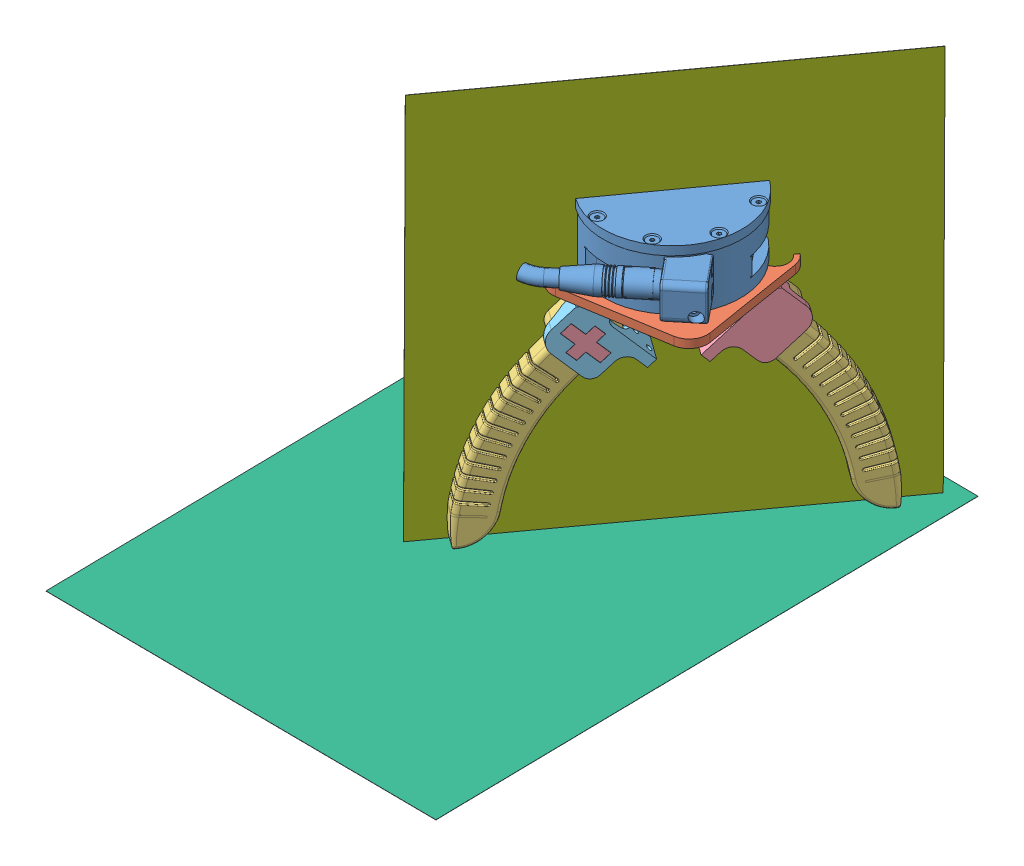
SolidWorks assembly Assem_ee, configuration Default. Lengths in mm.
Overall size (212.48 223.84 298.79).
58 component instances, 34 part files, 23 mates.
Components (placement in the parent):
- ati_gamma_sensor_mount _up-1: ati_gamma_sensor_mount _up [Default] at (-15.434 18.2375 114.8285) size (94 14.49 94) (hidden)
- ati_gamma_sensor_mount _down_L515-1: ati_gamma_sensor_mount _down_L515 [Default] at (-15.434 18.2375 114.8285) x (0 0 1) z (-1 0 0) size (114.18 58 114.18) (hidden)
- ATI-9105-TIF-GAMMA-1: ATI-9105-TIF-GAMMA [Default] at (-15.434 10.2375 114.8285) x (-0.987109 0 0.160048) z (0 1 0) size (81.43 106.62 33.32)
- fixture-1: fixture [Default] at (15.9943 -30.0869 71.2365) x (-0.987109 0 0.160048) z (0 1 0) size (76 76 7.57)
- Assem_soft-1: Assem_soft [Default] at (-95.8769 -63.8673 78.8152) x (0.181198 -0.950797 -0.251303) z (0.811158 0.000013 0.584827) size (139.54 63.23 30.2)
  - finger_proto_4.2-1: finger_proto_4.2 [Default] at (-2.494 64.561 95.5128) size (120.36 42.19 26.68)
  - linkag_3-1: linkag_3 [Default] at (-2.8273 57.773 71.3134) x (0.891388 0.453242 -0.000014) z (0.000014 0.000003 1) size (40.75 42 30.2)
  - linkage_4-1: linkage_4 [Default] at (-2.8273 57.773 71.3134) x (0.891388 0.453242 -0.000014) z (0.000014 0.000003 1) size (40.75 42 15)
- Assem_soft-2: Assem_soft [Default] at (65.1711 -63.8673 150.9587) x (-0.181198 -0.950797 0.251303) z (-0.811158 0.000013 -0.584827) size (139.54 63.23 30.2)
  - finger_proto_4.2-1: finger_proto_4.2 [Default] at (-2.494 64.561 95.5128) size (120.36 42.19 26.68)
  - linkag_3-1: linkag_3 [Default] at (-2.8273 57.773 71.3134) x (0.891388 0.453242 -0.000014) z (0.000014 0.000003 1) size (40.75 42 30.2)
  - linkage_4-1: linkage_4 [Default] at (-2.8273 57.773 71.3134) x (0.891388 0.453242 -0.000014) z (0.000014 0.000003 1) size (40.75 42 15)
- Assem1-1: Assem1 [Default] at (17.137 -120.8618 -18.1601) x (0.539853 0.425322 0.726403) z (-0.534722 0.839751 -0.094291) size (112.36 145.16 142) (hidden)
  - CAM holder (1)-1: CAM holder (1) [Default] at (82.7281 3.9301 79.7737) x (0.895378 -0.021687 -0.444779) z (0.425322 0.33752 0.839751) size (64.99 120.47 90)
  - Top CAM (1)-1: Top CAM (1) [Default] at (81.9279 129.0526 71.921) x (0.895378 -0.021687 -0.444779) z (-0.425322 -0.33752 -0.839751) size (65 111.17 15.1)
- Intel_RealSense_L515_CAD_external.stp-1: Intel_RealSense_L515_CAD_external.stp [Default] at (106.8055 -15.7625 -7.3222) x (-0.587716 0 -0.809067) z (0 -1 0) size (61.01 64.04 35.39) (hidden)
  - TA_PERIPHERAL_L515_ASM_25_ASM.stp-1: TA_PERIPHERAL_L515_ASM_25_ASM.stp [Default] at origin size (61.01 64.04 35.39)
    - CENTER_HEAT_SINK_SUBASM_L515_AS_ASM.stp-1: CENTER_HEAT_SINK_SUBASM_L515_AS_ASM.stp [Default] at origin size (26.06 28.22 15.92)
      - OPTICAL_HEAD_GEN_1_L515_ASM_6_ASM.stp-1: OPTICAL_HEAD_GEN_1_L515_ASM_6_ASM.stp [Default] at origin size (26.06 28.22 15.92)
        - RXFOV_72X60_P_040419_2.stp-1: RXFOV_72X60_P_040419_2.stp [Default] at (-18.5 -15 -9.623) size (26.06 21.31 15.92) (hidden)
        - TX_FOV_1_2_73X59_040419_2.stp-1: TX_FOV_1_2_73X59_040419_2.stp [Default] at (-18.5 -15 -9.623) size (19.97 16.11 9.45) (hidden)
    - FRONT_OPTICAL_ASSEMBLY_L515_ASM_ASM.stp-1: FRONT_OPTICAL_ASSEMBLY_L515_ASM_ASM.stp [Default] at origin size (24.45 11.78 6.27)
      - CAMERA_2MP_FF_OV2740_CMOS_ASM_1_ASM.stp-1: CAMERA_2MP_FF_OV2740_CMOS_ASM_1_ASM.stp [Default] at (0 0 -22.68) size (8 5.7 2.8)
        - L500_RGB_2MP_1_2_2.stp-1: L500_RGB_2MP_1_2_2.stp [Default] at origin size (8 5.7 2.8)
      - PCB_ASSY_RGB_INTERPOSER_L515_AS_ASM.stp-1: PCB_ASSY_RGB_INTERPOSER_L515_AS_ASM.stp [Default] at origin size (24.45 11.78 3.75)
        - RGB_INTERPOSER_AS03021_23AUG_7.stp-1: RGB_INTERPOSER_AS03021_23AUG_7.stp [Default] at (-14.55 7.36 -5.546) size (24.45 11.78 3.72)
        - KAPTON_RGB_INTERPOSER_L515_8.stp-1: KAPTON_RGB_INTERPOSER_L515_8.stp [Default] at origin size (20.84 11.78 0.05)
        - CONN_FPC_BTM_21POS_-3MM_PITCH_2.stp-1: CONN_FPC_BTM_21POS_-3MM_PITCH_2.stp [Default] at (11.985 13.432 -5.615) x (0 -1 0) z (1 0 0) size (7.5 0.9 2.83)
        - CONN_HEADER_3-0MM_20POS_PWR_2.stp-1: CONN_HEADER_3-0MM_20POS_PWR_2.stp [Default] at (-10.26 11.36 -5.58) x (0 -1 0) z (0 0 -1) size (5.9 2.35 2.24)
    - PCB_ASSEMBLY_MA_ASIC_L515_ASM_5_ASM.stp-1: PCB_ASSEMBLY_MA_ASIC_L515_ASM_5_ASM.stp [Default] at origin size (43.47 31.41 6.28)
      - L500_PCB_ASIC_BOARD_OCT08_ASM_1_ASM.stp-1: L500_PCB_ASIC_BOARD_OCT08_ASM_1_ASM.stp [Default] at (0 0 0.6) size (43.47 31.41 6.28)
        - A-PCB_ASIC_20_ASM_1_ASM_1_ASM.stp-1: A-PCB_ASIC_20_ASM_1_ASM_1_ASM.stp [Default] at origin size (43.47 31.41 6.28)
          - 2UB2C02-000111F_3D_USB_TYPE_C_1_ASM.stp-1: 2UB2C02-000111F_3D_USB_TYPE_C_1_ASM.stp [Default] at (-14.4895 -10.5138 -15.4) x (-0.58723 0.80942 0) z (0 0 -1) size (9.7 11.1 6.08)
            - 2UB2C02-000111F_3D_USB_TYPE_C_2.stp-1: 2UB2C02-000111F_3D_USB_TYPE_C_2.stp [Default] at origin size (9.7 11.1 6.08)
            - 2UB2C02-000111F_3D_USB_TYPE_C_3.stp-1: 2UB2C02-000111F_3D_USB_TYPE_C_3.stp [Default] at origin size (0.28 0.35 0.16)
          - P-PCB_ASIC_20_1_3.stp-1: P-PCB_ASIC_20_1_3.stp [Default] at origin size (41.95 30.8 1)
      - BM03B-SRSS-TB_1.stp-1: BM03B-SRSS-TB_1.stp [Default] at (15.2095 -11.0504 -16.2) x (0.587785 0.809017 0) z (0 0 -1) size (5 4.32 3.6)
    - REAR_HOUSING_ASSEMBLY_L515_ASM__ASM.stp-1: REAR_HOUSING_ASSEMBLY_L515_ASM__ASM.stp [Default] at origin size (61.01 64.04 26)
      - INTAKE_VENT_L515_9.stp-1: INTAKE_VENT_L515_9.stp [Default] at origin size (12.82 7.66 16.91)
      - INTAKE_VENT_L515_9.stp-2: INTAKE_VENT_L515_9.stp [Default] x (0.660526 0.750803 0) z (0 0 1) size (12.82 7.66 16.91)
      - REAR_HOUSING_L515_25.stp-1: REAR_HOUSING_L515_25.stp [Default] at origin size (61.01 61.01 26)
    - COVER_WINDOW_SUBASM_L515_ASM_2_ASM.stp-1: COVER_WINDOW_SUBASM_L515_ASM_2_ASM.stp [Default] at origin size (57.86 57.86 2.18)
      - COVER_WINDOW_IR_W_ADHESIVE_L515_ASM.stp-1: COVER_WINDOW_IR_W_ADHESIVE_L515_ASM.stp [Default] at origin size (57.86 57.86 0.78)
        - COVER_WINDOW_IR_L515_10.stp-1: COVER_WINDOW_IR_L515_10.stp [Default] at origin size (57.86 57.86 0.5)
        - COVER_WINDOW_MASK_L515_10.stp-1: COVER_WINDOW_MASK_L515_10.stp [Default] at origin size (57.56 57.56 0.03)
        - COVER_WINDOW_RGB_RING_L515_8.stp-1: COVER_WINDOW_RGB_RING_L515_8.stp [Default] at origin size (7.8 7.8 0.03)
        - ADHESIVE_COVER_WINDOW_IR_L515_1.stp-1: ADHESIVE_COVER_WINDOW_IR_L515_1.stp [Default] at origin size (57.36 57.36 0.25)
      - FOAM_ISOLATION_RGB_L515_ASM_15_ASM.stp-1: FOAM_ISOLATION_RGB_L515_ASM_15_ASM.stp [Default] at origin size (18 37.16 1.6)
        - FOAM_ISOLATION_RGB_L515_13.stp-1: FOAM_ISOLATION_RGB_L515_13.stp [Default] at origin size (18 37.16 1.5)
        - ADHESIVE_ISOLATION_RGB_L515_11.stp-1: ADHESIVE_ISOLATION_RGB_L515_11.stp [Default] at origin size (18 37.16 0.1)
      - COVER_WINDOW_SLOT_FILLER_L515_8.stp-1: COVER_WINDOW_SLOT_FILLER_L515_8.stp [Default] at origin size (15.1 1.1 0.5)
      - FOAM_SEALING_CW_FHS_L515_16.stp-1: FOAM_SEALING_CW_FHS_L515_16.stp [Default] at origin size (39.78 43.86 1.4)
    - AUX_DOOR_ASSEMBLY_L515_ASM_7_ASM.stp-1: AUX_DOOR_ASSEMBLY_L515_ASM_7_ASM.stp [Default] at origin size (9.18 11.47 3.61)
      - AUX_DOOR_L515_8.stp-1: AUX_DOOR_L515_8.stp [Default] at origin size (9.18 11.47 3.61)
      - STEEL_PIN_2.stp-1: STEEL_PIN_2.stp [Default] at (25.6249 -13.3025 -17.25) x (-0.587785 -0.809017 0) z (-0.809017 0.587785 0) size (1.6 1.6 1.6)
      - STEEL_PIN_2.stp-2: STEEL_PIN_2.stp [Default] at (20.57 -20.26 -17.25) x (-0.587785 -0.809017 0) z (-0.809017 0.587785 0) size (1.6 1.6 1.6)
- A4 paper-1: A4 paper [Default] at (59.757 -146.945 318.5652) x (-0.999818 0.017006 0.008599) z (0.008459 -0.008282 0.99993) size (210 0.1 297)
- frame-1: frame [Default] at (-76.5084 -143.65 199.8824) x (0.001981 0.999994 -0.002747) z (-0.584817 0.003387 0.811158) size (210 0.1 210)
Mates (geometry in assembly coordinates):
- Coincident1: coincident anti-aligned: plane of ati_gamma_sensor_mount _up-1 through (-15.434 18.2375 114.8285) normal (0 -1 0); plane of ati_gamma_sensor_mount _down_L515-1 through (-15.434 18.2375 114.8285) normal (0 1 0)
- Coincident4: coincident anti-aligned: plane of ati_gamma_sensor_mount _down_L515-1 through (-15.434 10.2375 114.8285) normal (0 -1 0); plane of ATI-9105-TIF-GAMMA-1 through (-15.434 10.2375 114.8285) normal (0 1 0)
- Coincident8: coincident anti-aligned: plane of ATI-9105-TIF-GAMMA-1 through (-15.434 -23.0869 114.8285) normal (0 -1 0); plane of fixture-1 through (-15.434 -23.0869 114.8285) normal (0 1 0)
- Concentric3: concentric aligned: cylinder of ATI-9105-TIF-GAMMA-1 through (-0.8135 -17.4869 94.5494) axis (0 -1 0) radius 2.5502; cylinder of fixture-1 through (-0.8135 -26.2869 94.5494) axis (0 -1 0) radius 7.25
- Concentric4: concentric anti-aligned: cylinder of ATI-9105-TIF-GAMMA-1 through (-30.0545 -17.4869 135.1075) axis (0 -1 0) radius 2.5502; cylinder of fixture-1 through (-30.0545 -30.0869 135.1075) axis (0 1 0) radius 3.1
- Concentric5: concentric aligned: cylinder of fixture-1 through (-13.83 -30.0869 93.7945) axis (0 1 0) radius 1.575; cylinder of Assem_soft-1/linkage_4-1 through (-13.83 -38.0869 93.7945) axis (0 1 0) radius 1.5
- Concentric6: concentric aligned: cylinder of fixture-1 through (4.1778 -30.0869 106.7775) axis (0 1 0) radius 1.575; cylinder of Assem_soft-1/linkag_3-1 through (4.1778 -38.0869 106.7775) axis (0 1 0) radius 1.5
- Coincident9: coincident anti-aligned: plane of fixture-1 through (15.9943 -30.0869 71.2365) normal (0 -1 0); plane of Assem_soft-1/linkag_3-1 through (-1.991 -30.0869 108.4941) normal (0 1 0)
- Coincident10: coincident anti-aligned: plane of fixture-1 through (15.9943 -30.0869 71.2365) normal (0 -1 0); plane of Assem_soft-2/linkag_3-1 through (-28.7148 -30.0869 121.2799) normal (0 1 0)
- Concentric7: concentric aligned: cylinder of fixture-1 through (-34.8836 -30.0869 122.9964) axis (0 1 0) radius 1.575; cylinder of Assem_soft-2/linkag_3-1 through (-34.8836 -38.0869 122.9964) axis (0 1 0) radius 1.5
- Concentric8: concentric aligned: circle of fixture-1; cylinder of Assem_soft-2/linkage_4-1 through (-16.8758 -38.0869 135.9794) axis (0 1 0) radius 1.5
- Coincident11: coincident anti-aligned: plane of ati_gamma_sensor_mount _down_L515-1 through (51.7411 10.2375 61.7955) normal (0.707107 0 -0.707107); plane of Assem1-1/CAM holder (1)-1 through (21.6891 -17.3593 31.7434) normal (-0.707107 0 0.707107)
- Concentric9: concentric anti-aligned: cylinder of ati_gamma_sensor_mount _down_L515-1 through (39.0132 60.2375 60.3813) axis (0.707107 0 -0.707107) radius 3.05; circle of Assem1-1/CAM holder (1)-1
- Parallel1: parallel anti-aligned: plane of fixture-1 through (15.9943 -30.0869 71.2365) normal (0 -1 0); plane of Intel_RealSense_L515_CAD_external.stp-1/TA_PERIPHERAL_L515_ASM_25_ASM.stp-1/REAR_HOUSING_ASSEMBLY_L515_ASM__ASM.stp-1/REAR_HOUSING_L515_25.stp-1 through (106.8055 10.2375 -7.3222) normal (0 1 0)
- Coincident13: coincident anti-aligned: plane of ati_gamma_sensor_mount _down_L515-1 through (-15.434 10.2375 114.8285) normal (0 -1 0); plane of Intel_RealSense_L515_CAD_external.stp-1/TA_PERIPHERAL_L515_ASM_25_ASM.stp-1/REAR_HOUSING_ASSEMBLY_L515_ASM__ASM.stp-1/REAR_HOUSING_L515_25.stp-1 through (106.8055 10.2375 -7.3222) normal (0 1 0)
- Concentric10: concentric anti-aligned: cylinder of ati_gamma_sensor_mount _down_L515-1 through (39.0132 30.2375 60.3813) axis (0.707107 0 -0.707107) radius 3.05; circle of Assem1-1/CAM holder (1)-1
- Coincident14: coincident aligned: plane of ati_gamma_sensor_mount _up-1 through (31.566 26.2375 67.8285) normal (1 0 0); plane of ati_gamma_sensor_mount _down_L515-1 through (31.566 10.2375 67.8285) normal (1 0 0)
- Concentric11: concentric aligned: cylinder of ati_gamma_sensor_mount _up-1 through (-53.434 18.2375 76.8285) axis (0 1 0) radius 3.1; cylinder of ati_gamma_sensor_mount _down_L515-1 through (-53.434 10.2375 76.8285) axis (0 1 0) radius 3.1
- Concentric13: concentric aligned: cylinder of Assem1-1/Top CAM (1)-1 through (106.8055 14.9375 -7.3222) axis (0 -1 0) radius 9.8; cylinder of Intel_RealSense_L515_CAD_external.stp-1/TA_PERIPHERAL_L515_ASM_25_ASM.stp-1/REAR_HOUSING_ASSEMBLY_L515_ASM__ASM.stp-1/REAR_HOUSING_L515_25.stp-1 through (106.8055 11.5375 -7.3222) axis (0 -1 0) radius 30.5
- Coincident16: coincident anti-aligned: plane of ati_gamma_sensor_mount _down_L515-1 through (-15.434 10.2375 114.8285) normal (0 -1 0); plane of ATI-9105-TIF-GAMMA-1 through (-15.434 10.2375 114.8285) normal (0 1 0)
- Concentric14: concentric anti-aligned: cylinder of ati_gamma_sensor_mount _up-1 through (-15.434 32.6375 114.8285) axis (0 -1 0) radius 40; cylinder of ATI-9105-TIF-GAMMA-1 through (-15.434 5.5131 114.8285) axis (0 1 0) radius 37.719
- Coincident24: coincident anti-aligned: plane of frame-1 through (-76.5896 -143.65 199.8239) normal (-0.811163 0 -0.584821)
- Coincident25: coincident: plane of A4 paper-1 through (59.757 -146.945 318.5652) normal (0.017076 0.999821 0.008137); line of frame-1 through (46.2221 -144.3613 29.4807) axis (-0.584817 0.003387 0.811158)
